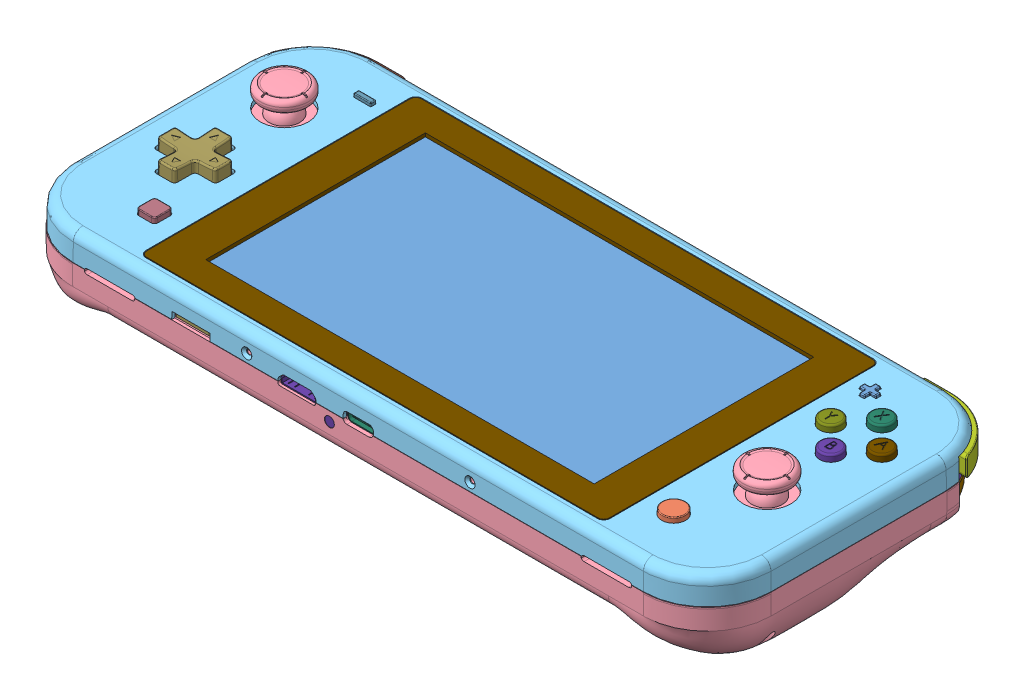
SolidWorks assembly Assembly Retro Lite CM5_1, configuration Default. Lengths in mm. (continued)
Components (placement in the parent): (continued)
- Assembly Center Components-1: Assembly Center Components [Default] at (0 9.4999 0) size (146.77 13.35 93.89) (continued)
  - Radxa CM3-1: Radxa CM3 [Default] at (-34.1679 -8.7691 -17.6603) x (0 0 -1) z (0 -1 0) size (40.05 55.02 3.7) (continued)
    - EMP_Models-1: EMP_Models [Default] at origin size (39.5 54.73 3.7) (continued)
      - C10-146: C10 [Default] at (-1.1975 3.8019 -1.2) x (-0.707107 -0.707107 0) z (0 0 -1) size (1.1 0.6 0.35)
      - C105-44: C105 [Default] at (-1.5975 -0.3481 -1.2) x (0.707107 0.707107 0) z (0 0 -1) size (2.5 1.3 0.6)
      - C10-147: C10 [Default] at (1.95 -3.55 -1.2) x (-0.707107 -0.707107 0) z (0 0 -1) size (1.1 0.6 0.35)
      - C10-148: C10 [Default] at (2.3 -3.9 -1.2) x (-0.707107 -0.707107 0) z (0 0 -1) size (1.1 0.6 0.35)
      - C10-149: C10 [Default] at (-1.7 4.85 -1.2) x (-0.707107 -0.707107 0) z (0 0 -1) size (1.1 0.6 0.35)
      - C10-150: C10 [Default] at (-0.45 4.65 -1.2) x (0.707107 -0.707107 0) z (0 0 -1) size (1.1 0.6 0.35)
      - C10-151: C10 [Default] at (-14.45 -16.6 -1.2) x (1 0 0) z (0 0 -1) size (1.1 0.6 0.35)
      - C10-152: C10 [Default] at (-5.6475 1.4519 -1.2) x (-0.707107 -0.707107 0) z (0 0 -1) size (1.1 0.6 0.35)
      - C10-153: C10 [Default] at (-9.5877 22.6017 0) x (0 1 0) z (0 0 1) size (1.1 0.6 0.35)
      - C10-154: C10 [Default] at (-4.9838 2.7384 -1.2) x (-0.707107 -0.707107 0) z (0 0 -1) size (1.1 0.6 0.35)
      - C10-155: C10 [Default] at (-3.4533 2.4614 -1.2) x (0.707107 0.707107 0) z (0 0 -1) size (1.1 0.6 0.35)
      - C10-156: C10 [Default] at (-4.2975 3.6019 -1.2) x (-0.707107 0.707107 0) z (0 0 -1) size (1.1 0.6 0.35)
      - C10-157: C10 [Default] at (1.6525 -1.6481 -1.2) x (-0.707107 -0.707107 0) z (0 0 -1) size (1.1 0.6 0.35)
      - C10-158: C10 [Default] at (0.25 10.55 -1.2) x (0 1 0) z (0 0 -1) size (1.1 0.6 0.35)
      - C10-159: C10 [Default] at (-5.2818 15.3952 0) size (1.1 0.6 0.35)
      - C10-160: C10 [Default] at (3.4025 -2.2481 -1.2) x (0.707107 0.707107 0) z (0 0 -1) size (1.1 0.6 0.35)
      - C10-161: C10 [Default] at (2.8025 -1.6481 -1.2) x (-0.707107 0.707107 0) z (0 0 -1) size (1.1 0.6 0.35)
      - C10-162: C10 [Default] at (-6.7675 7.1519 0) x (-0.707107 0.707107 0) z (0 0 1) size (1.1 0.6 0.35)
      - C10-163: C10 [Default] at (-6.3865 7.5329 0) x (-0.707107 0.707107 0) z (0 0 1) size (1.1 0.6 0.35)
      - C10-164: C10 [Default] at (8.6535 15.7139 -1.2) x (-1 0 0) z (0 0 -1) size (1.1 0.6 0.35)
      - C10-165: C10 [Default] at (-5.4975 8.5489 0) x (-0.707107 0.707107 0) z (0 0 1) size (1.1 0.6 0.35)
      - C10-166: C10 [Default] at (-5.9125 8.0719 0) x (-0.707107 0.707107 0) z (0 0 1) size (1.1 0.6 0.35)
      - C10-167: C10 [Default] at (-2.6475 4.9519 -1.2) x (0.707107 -0.707107 0) z (0 0 -1) size (1.1 0.6 0.35)
      - C1-22: C1 [Default] at (0.2025 -1.3981 -1.2) x (-0.707107 -0.707107 0) z (0 0 -1) size (1.7 0.9 0.5)
      - C10-168: C10 [Default] at (2.0525 -2.0981 -1.2) x (0.707107 0.707107 0) z (0 0 -1) size (1.1 0.6 0.35)
      - C1-23: C1 [Default] at (8.3303 14.9277 -1.2) x (-1 0 0) z (0 0 -1) size (1.7 0.9 0.5)
      - C1-24: C1 [Default] at (0.9 11.1 -1.2) x (0 1 0) z (0 0 -1) size (1.7 0.9 0.5)
      - C10-169: C10 [Default] at (-12.4547 0.1177 0) x (0.707107 -0.707107 0) z (0 0 1) size (1.1 0.6 0.35)
      - C10-170: C10 [Default] at (-12.9047 -0.3323 0) x (0.707107 -0.707107 0) z (0 0 1) size (1.1 0.6 0.35)
      - C10-171: C10 [Default] at (-6.4948 1.7665 -1.2) x (0.707107 -0.707107 0) z (0 0 -1) size (1.1 0.6 0.35)
      - C10-172: C10 [Default] at (-9.7716 0.8527 -1.2) x (-1 0 0) z (0 0 -1) size (1.1 0.6 0.35)
      - C10-173: C10 [Default] at (-7.95 1 -1.2) x (-0.707107 0.707107 0) z (0 0 -1) size (1.1 0.6 0.35)
      - C10-174: C10 [Default] at (-9.7407 -1.0384 -1.2) x (-1 0 0) z (0 0 -1) size (1.1 0.6 0.35)
      - C10-175: C10 [Default] at (-5.8561 -0.2604 -1.2) x (-0.707107 -0.707107 0) z (0 0 -1) size (1.1 0.6 0.35)
      - C1-25: C1 [Default] at (1.8025 -0.5481 -1.2) x (0.707107 0.707107 0) z (0 0 -1) size (1.7 0.9 0.5)
      - C10-176: C10 [Default] at (-5.0975 0.5019 -1.2) x (-0.707107 0.707107 0) z (0 0 -1) size (1.1 0.6 0.35)
      - C10-177: C10 [Default] at (2.5525 1.6519 -1.2) x (0.707107 0.707107 0) z (0 0 -1) size (1.1 0.6 0.35)
      - C10-178: C10 [Default] at (11.45 15.45 -1.2) x (0 1 0) z (0 0 -1) size (1.1 0.6 0.35)
      - C10-179: C10 [Default] at (2.7525 3.1519 -1.2) x (0.707107 0.707107 0) z (0 0 -1) size (1.1 0.6 0.35)
      - C10-180: C10 [Default] at (1.5525 2.5519 -1.2) x (0.707107 0.707107 0) z (0 0 -1) size (1.1 0.6 0.35)
      - C1-26: C1 [Default] at (13.7559 7.4017 0) size (1.7 0.9 0.5)
      - C10-181: C10 [Default] at (14.0564 10.6567 -1.2) x (0 1 0) z (0 0 -1) size (1.1 0.6 0.35)
      - C10-182: C10 [Default] at (14.055 9.1901 -1.2) x (0 -1 0) z (0 0 -1) size (1.1 0.6 0.35)
      - C10-183: C10 [Default] at (4.1525 -1.7481 -1.2) x (0.707107 -0.707107 0) z (0 0 -1) size (1.1 0.6 0.35)
      - C10-184: C10 [Default] at (2.0525 3.8519 -1.2) x (0.707107 0.707107 0) z (0 0 -1) size (1.1 0.6 0.35)
      - C1-27: C1 [Default] at (-0.4475 -0.7481 -1.2) x (-0.707107 -0.707107 0) z (0 0 -1) size (1.7 0.9 0.5)
      - C10-185: C10 [Default] at (-4.6 2.4 -1.2) x (-0.707107 -0.707107 0) z (0 0 -1) size (1.1 0.6 0.35)
      - C10-186: C10 [Default] at (2.4025 3.5019 -1.2) x (0.707107 0.707107 0) z (0 0 -1) size (1.1 0.6 0.35)
      - C10-187: C10 [Default] at (1.9025 2.2019 -1.2) x (0.707107 0.707107 0) z (0 0 -1) size (1.1 0.6 0.35)
      - C10-188: C10 [Default] at (1.1525 4.7519 -1.2) x (0.707107 0.707107 0) z (0 0 -1) size (1.1 0.6 0.35)
      - C10-189: C10 [Default] at (-10.8073 4.7134 0) x (-0.707107 0.707107 0) z (0 0 1) size (1.1 0.6 0.35)
      - C10-190: C10 [Default] at (-10.3573 5.1634 0) x (-0.707107 0.707107 0) z (0 0 1) size (1.1 0.6 0.35)
      - C10-191: C10 [Default] at (-9.9183 5.6024 0) x (-0.707107 0.707107 0) z (0 0 1) size (1.1 0.6 0.35)
      - C10-192: C10 [Default] at (-9.4886 6.0727 0) x (-0.707107 0.707107 0) z (0 0 1) size (1.1 0.6 0.35)
      - C10-193: C10 [Default] at (-8.5795 5.5319 0) x (-0.707107 0.707107 0) z (0 0 1) size (1.1 0.6 0.35)
      - C10-194: C10 [Default] at (-8.1985 5.9129 0) x (-0.707107 0.707107 0) z (0 0 1) size (1.1 0.6 0.35)
      - C105-45: C105 [Default] at (9.65 11.1 -1.2) x (-1 0 0) z (0 0 -1) size (2.5 1.3 0.6)
      - C10-195: C10 [Default] at (-7.2405 6.7439 0) x (-0.707107 0.707107 0) z (0 0 1) size (1.1 0.6 0.35)
      - C10-196: C10 [Default] at (-7.6905 6.2939 0) x (-0.707107 0.707107 0) z (0 0 1) size (1.1 0.6 0.35)
      - C10-197: C10 [Default] at (0.0606 6.505 -1.2) x (1 0 0) z (0 0 -1) size (1.1 0.6 0.35)
      - C10-198: C10 [Default] at (1.6025 4.3019 -1.2) x (0.707107 0.707107 0) z (0 0 -1) size (1.1 0.6 0.35)
      - C10-199: C10 [Default] at (0.45 4.15 -1.2) x (-0.707107 0.707107 0) z (0 0 -1) size (1.1 0.6 0.35)
      - C10-200: C10 [Default] at (4.3525 1.0519 -1.2) x (-0.707107 -0.707107 0) z (0 0 -1) size (1.1 0.6 0.35)
      - C10-201: C10 [Default] at (-0.25 3.6 -1.2) x (-0.707107 -0.707107 0) z (0 0 -1) size (1.1 0.6 0.35)
      - C10-202: C10 [Default] at (-4.7475 1.3019 -1.2) x (-0.707107 -0.707107 0) z (0 0 -1) size (1.1 0.6 0.35)
      - C10-203: C10 [Default] at (0.9 2.95 -1.2) x (0.707107 -0.707107 0) z (0 0 -1) size (1.1 0.6 0.35)
      - C10-204: C10 [Default] at (4.05 11.1 -1.2) x (0 -1 0) z (0 0 -1) size (1.1 0.6 0.35)
      - D1-1: D1 [Default] at (13.3703 9.2021 0) x (-1 0 0) z (0 0 1) size (3.3 1.4 0.8)
      - D1-2: D1 [Default] at (15.4253 4.4887 0) x (0 -1 0) z (0 0 1) size (3.3 1.4 0.8)
      - ED8144-1: ED8144 [Default] at (-15.7 3.95 0) x (0 1 0) z (0 0 1) size (1.77 0.93 0.8)
      - ED8144-2: ED8144 [Default] at (-14.65 -20.2 0) size (1.77 0.93 0.8)
      - ED8144-3: ED8144 [Default] at (-2.4887 24.0177 0) x (0 1 0) z (0 0 1) size (1.77 0.93 0.8)
      - ED8147-1: ED8147 [Default] at (18.2193 9.1971 0) size (2.41 1.24 0.8)
      - ED8144-4: ED8144 [Default] at (17.6586 1.0982 0) x (0 -1 0) z (0 0 1) size (1.77 0.93 0.8)
      - ED8144-5: ED8144 [Default] at (17.6586 2.8762 0) x (0 1 0) z (0 0 1) size (1.77 0.93 0.8)
      - FB1-1: FB1 [Default] at (1.65 9.65 -1.2) x (1 0 0) z (0 0 -1) size (1.7 0.8 0.5)
      - FB1-2: FB1 [Default] at (9.4715 23.3369 0) x (0 1 0) z (0 0 1) size (1.7 0.8 0.5)
      - FB1-3: FB1 [Default] at (10.7443 20.4739 -1.2) x (1 0 0) z (0 0 -1) size (1.7 0.8 0.5)
      - FB1-4: FB1 [Default] at (9.7417 13.5389 -1.2) x (1 0 0) z (0 0 -1) size (1.7 0.8 0.5)
      - FB1-5: FB1 [Default] at (12.05 13.95 -1.2) x (0 -1 0) z (0 0 -1) size (1.7 0.8 0.5)
      - FB1-6: FB1 [Default] at (3.5025 2.1519 -1.2) x (-0.707107 0.707107 0) z (0 0 -1) size (1.7 0.8 0.5)
      - FB5-1: FB5 [Default] at (17.7525 -10.7981 0) x (0 -1 0) z (0 0 1) size (2.08 1.34 0.7)
      - FB5-2: FB5 [Default] at (16.3025 -10.7981 0) x (0 -1 0) z (0 0 1) size (2.08 1.34 0.7)
      - FB5-3: FB5 [Default] at (14.8525 -10.7981 0) x (0 -1 0) z (0 0 1) size (2.08 1.34 0.7)
      - FB5-4: FB5 [Default] at (13.4025 -10.7981 0) x (0 -1 0) z (0 0 1) size (2.08 1.34 0.7)
      - FB9-1: FB9 [Default] at (11.1972 22.9552 0) size (2.8 1.3 0.6)
      - J1-1: J1 [Default] at (11.3212 22.5507 -1.2) x (0 1 0) z (0 0 -1) size (2.84 22.55 1)
      - J90033-1: J90033 [Default] at (-13.7 5.05 0) x (0 1 0) z (0 0 1) size (4.08 2.13 0.5)
      - J90033-2: J90033 [Default] at (-16.8 -18.5 0) x (-1 0 0) z (0 0 1) size (4.08 2.13 0.5)
      - L1-1: L1 [Default] at (9.3525 -25.5481 0) x (0 1 0) z (0 0 1) size (2.78 2.28 1)
      - L10-1: L10 [Default] at (5.8 11.7 0) x (0 1 0) z (0 0 1) size (2.78 2.28 1)
      - L10-2: L10 [Default] at (12.0115 18.7649 0) size (2.78 2.28 1)
      - L10-3: L10 [Default] at (-0.9 20.75 0) x (0 1 0) z (0 0 1) size (2.78 2.28 1)
      - L13-1: L13 [Default] at (-13.7665 -4.2312 0) x (-0.707107 -0.707107 0) z (0 0 1) size (2.83 2.1 1.2)
      - L2-1: L2 [Default] at (-11.1177 21.5067 0) x (-0.707107 -0.707107 0) z (0 0 1) size (1.1 0.6 0.35)
      - L2-2: L2 [Default] at (-11.7527 23.4117 0) x (-1 0 0) z (0 0 1) size (1.1 0.6 0.35)
      - L10-4: L10 [Default] at (-17.3475 4.7519 0) x (0 -1 0) z (0 0 1) size (2.78 2.28 1)
      - L10-5: L10 [Default] at (18.3025 -19.6481 0) x (-1 0 0) z (0 0 1) size (2.78 2.28 1)
      - L10-6: L10 [Default] at (9.2 12.15 0) x (-1 0 0) z (0 0 1) size (2.78 2.28 1)
      - L10-7: L10 [Default] at (-0.85 16.7 0) x (0 1 0) z (0 0 1) size (2.78 2.28 1)
      - LED1-1: LED1 [Default] at (-2.8224 26.4941 0) x (-1 0 0) z (0 0 1) size (2.95 1.43 0.6)
      - M1-1: M1 [Default] at (-12.0975 -25.5981 -1.2) x (-1 0 0) z (0 0 -1) size (3.45 3.45 0.1)
      - M1-2: M1 [Default] at (12.2025 25.6519 0) size (3.45 3.45 0.1)
      - M1-3: M1 [Default] at (-12.0975 -25.5981 0) size (3.45 3.45 0.1)
      - M1-4: M1 [Default] at (12.2025 25.6519 -1.2) x (-1 0 0) z (0 0 -1) size (3.45 3.45 0.1)
      - Q4-1: Q4 [Default] at (-8.45 5.5 -1.2) x (-1 0 0) z (0 0 -1) size (1.27 1.32 0.8)
      - Q5-1: Q5 [Default] at (-7.3 23.05 0) size (3.35 3.3 1)
      - Q5-2: Q5 [Default] at (17 -3.9 0) x (-1 0 0) z (0 0 1) size (3.35 3.3 1)
      - R1-1: R1 [Default] at (6.8025 -4.5481 -1.2) x (1 0 0) z (0 0 -1) size (1.7 0.9 0.5)
      - L2-3: L2 [Default] at (12.9303 4.6718 -1.2) x (0 -1 0) z (0 0 -1) size (1.1 0.6 0.35)
      - L2-4: L2 [Default] at (17.75 -11.3 -1.2) x (0 1 0) z (0 0 -1) size (1.1 0.6 0.35)
      - L2-5: L2 [Default] at (17.75 -12.45 -1.2) x (0 1 0) z (0 0 -1) size (1.1 0.6 0.35)
      - L2-6: L2 [Default] at (15.7025 -17.9981 -1.2) x (0 1 0) z (0 0 -1) size (1.1 0.6 0.35)
      - L2-7: L2 [Default] at (18.45 -11.3 -1.2) x (0 1 0) z (0 0 -1) size (1.1 0.6 0.35)
      - L2-8: L2 [Default] at (18.45 -12.45 -1.2) x (0 1 0) z (0 0 -1) size (1.1 0.6 0.35)
      - L2-9: L2 [Default] at (15.0525 -17.9981 -1.2) x (0 1 0) z (0 0 -1) size (1.1 0.6 0.35)
      - L2-10: L2 [Default] at (15.0525 -19.1481 -1.2) x (0 1 0) z (0 0 -1) size (1.1 0.6 0.35)
      - L2-11: L2 [Default] at (13.7525 -17.9981 -1.2) x (0 1 0) z (0 0 -1) size (1.1 0.6 0.35)
      - L2-12: L2 [Default] at (13.7525 -19.1481 -1.2) x (0 1 0) z (0 0 -1) size (1.1 0.6 0.35)
      - R1-2: R1 [Default] at (12.7025 -9.6481 0) size (1.7 0.9 0.5)
      - L2-13: L2 [Default] at (0.4486 12.9437 -1.2) x (0 1 0) z (0 0 -1) size (1.1 0.6 0.35)
      - R1-3: R1 [Default] at (13.1025 -8.2481 0) x (0 -1 0) z (0 0 1) size (1.7 0.9 0.5)
      - L2-14: L2 [Default] at (14.4025 -17.9981 -1.2) x (0 1 0) z (0 0 -1) size (1.1 0.6 0.35)
      - L2-15: L2 [Default] at (14.4025 -19.1481 -1.2) x (0 1 0) z (0 0 -1) size (1.1 0.6 0.35)
      - R1-4: R1 [Default] at (12.9525 -11.8481 -1.2) x (-1 0 0) z (0 0 -1) size (1.7 0.9 0.5)
      - R1-5: R1 [Default] at (18.8525 -19.1481 -1.2) x (-1 0 0) z (0 0 -1) size (1.7 0.9 0.5)
      - L2-16: L2 [Default] at (11.8525 -13.8481 -1.2) x (0 -1 0) z (0 0 -1) size (1.1 0.6 0.35)
      - L2-17: L2 [Default] at (11.6025 -15.0981 -1.2) x (1 0 0) z (0 0 -1) size (1.1 0.6 0.35)
      - L2-18: L2 [Default] at (11.2025 -13.8481 -1.2) x (0 -1 0) z (0 0 -1) size (1.1 0.6 0.35)
      - L2-19: L2 [Default] at (11.7525 -16.2481 -1.2) x (-1 0 0) z (0 0 -1) size (1.1 0.6 0.35)
      - L2-20: L2 [Default] at (13.9025 -20.1981 0) x (0 -1 0) z (0 0 1) size (1.1 0.6 0.35)
      - R1-6: R1 [Default] at (11.8808 6.1274 0) size (1.7 0.9 0.5)
      - R1-7: R1 [Default] at (10.5014 7.0239 0) x (0 1 0) z (0 0 1) size (1.7 0.9 0.5)
      - L2-21: L2 [Default] at (-10.0048 -2.9217 0) x (-1 0 0) z (0 0 1) size (1.1 0.6 0.35)
      - L2-22: L2 [Default] at (-11.25 4.25 0) x (-0.707107 0.707107 0) z (0 0 1) size (1.1 0.6 0.35)
      - L2-23: L2 [Default] at (-7.55 2.1989 -1.2) x (1 0 0) z (0 0 -1) size (1.1 0.6 0.35)
      - L2-24: L2 [Default] at (18.2 -17.4 -1.2) x (-1 0 0) z (0 0 -1) size (1.1 0.6 0.35)
      - L2-25: L2 [Default] at (18.2 -16.75 -1.2) x (-1 0 0) z (0 0 -1) size (1.1 0.6 0.35)
      - L2-26: L2 [Default] at (19.25 -17.15 -1.2) x (0 -1 0) z (0 0 -1) size (1.1 0.6 0.35)
      - L2-27: L2 [Default] at (-13.3547 0.5177 0) x (-0.707107 -0.707107 0) z (0 0 1) size (1.1 0.6 0.35)
      - L2-28: L2 [Default] at (-3.95 9.75 0) x (0.707107 0.707107 0) z (0 0 1) size (1.1 0.6 0.35)
      - L2-29: L2 [Default] at (-7.45 4.9 -1.2) x (0 1 0) z (0 0 -1) size (1.1 0.6 0.35)
      - L2-30: L2 [Default] at (-3.35 10.8 0) x (0 1 0) z (0 0 1) size (1.1 0.6 0.35)
      - L2-31: L2 [Default] at (-8.9 -1.05 -1.2) x (0 1 0) z (0 0 -1) size (1.1 0.6 0.35)
      - L2-32: L2 [Default] at (-9.7407 -0.3884 -1.2) x (-1 0 0) z (0 0 -1) size (1.1 0.6 0.35)
      - L2-33: L2 [Default] at (1.5025 -5.4481 -1.2) x (-0.707107 -0.707107 0) z (0 0 -1) size (1.1 0.6 0.35)
      - L2-34: L2 [Default] at (-9.7625 1.3757 -1.2) x (1 0 0) z (0 0 -1) size (1.1 0.6 0.35)
      - L2-35: L2 [Default] at (-9.7722 0.251 -1.2) x (1 0 0) z (0 0 -1) size (1.1 0.6 0.35)
      - L2-36: L2 [Default] at (8.8525 -3.8481 -1.2) x (1 0 0) z (0 0 -1) size (1.1 0.6 0.35)
      - L2-37: L2 [Default] at (8.8525 -4.4981 -1.2) x (1 0 0) z (0 0 -1) size (1.1 0.6 0.35)
      - R24-1: R24 [Default] at (13.5019 5.7507 0) x (0 -1 0) z (0 0 1) size (2.5 1.3 0.6)
      - L2-38: L2 [Default] at (8.8525 -5.1481 -1.2) x (1 0 0) z (0 0 -1) size (1.1 0.6 0.35)
      - R1-8: R1 [Default] at (11.8808 7.9054 0) x (-1 0 0) z (0 0 1) size (1.7 0.9 0.5)
      - L2-39: L2 [Default] at (8.839 -5.6572 -1.2) x (-1 0 0) z (0 0 -1) size (1.1 0.6 0.35)
      - L2-40: L2 [Default] at (13.5019 8.1637 0) size (1.1 0.6 0.35)
      - R1-9: R1 [Default] at (11.8808 7.0164 0) x (-1 0 0) z (0 0 1) size (1.7 0.9 0.5)
      - L2-41: L2 [Default] at (1.9025 -4.5981 -1.2) x (-0.707107 0.707107 0) z (0 0 -1) size (1.1 0.6 0.35)
      - R1-10: R1 [Default] at (12.4 10.2 -1.2) x (-1 0 0) z (0 0 -1) size (1.7 0.9 0.5)
      - R1-11: R1 [Default] at (12.4278 9.235 -1.2) x (-1 0 0) z (0 0 -1) size (1.7 0.9 0.5)
      - L2-42: L2 [Default] at (0.0025 12.7519 0) x (0.707107 0.707107 0) z (0 0 1) size (1.1 0.6 0.35)
      - L2-43: L2 [Default] at (0.4393 12.3013 0) x (0.707107 0.707107 0) z (0 0 1) size (1.1 0.6 0.35)
      - L2-44: L2 [Default] at (0.9525 11.8019 0) x (0.707107 0.707107 0) z (0 0 1) size (1.1 0.6 0.35)
      - L2-45: L2 [Default] at (1.3881 11.3747 0) x (0.707107 0.707107 0) z (0 0 1) size (1.1 0.6 0.35)
      - L2-46: L2 [Default] at (1.9025 10.8519 0) x (0.707107 0.707107 0) z (0 0 1) size (1.1 0.6 0.35)
      - L2-47: L2 [Default] at (2.3296 10.4351 0) x (0.707107 0.707107 0) z (0 0 1) size (1.1 0.6 0.35)
      - L2-48: L2 [Default] at (2.8525 9.9019 0) x (0.707107 0.707107 0) z (0 0 1) size (1.1 0.6 0.35)
      - L2-49: L2 [Default] at (3.2748 9.4731 0) x (0.707107 0.707107 0) z (0 0 1) size (1.1 0.6 0.35)
      - L2-50: L2 [Default] at (-4.75 10.35 0) x (-1 0 0) z (0 0 1) size (1.1 0.6 0.35)
      - L2-51: L2 [Default] at (1.1909 6.5961 -1.2) x (0 -1 0) z (0 0 -1) size (1.1 0.6 0.35)
      - L2-52: L2 [Default] at (10.3525 2.1019 0) x (-0.707107 0.707107 0) z (0 0 1) size (1.1 0.6 0.35)
      - R1-12: R1 [Default] at (9.9432 9.4653 0) size (1.7 0.9 0.5)
      - R1-13: R1 [Default] at (9.5622 8.0683 0) x (0 -1 0) z (0 0 1) size (1.7 0.9 0.5)
      - L2-53: L2 [Default] at (-8.7065 -3.7391 0) size (1.1 0.6 0.35)
      - L2-54: L2 [Default] at (-8.7065 -4.3741 0) size (1.1 0.6 0.35)
      - L2-55: L2 [Default] at (-6.5975 -2.9981 -1.2) x (-0.707107 -0.707107 0) z (0 0 -1) size (1.1 0.6 0.35)
      - R1-14: R1 [Default] at (-15.4372 0.8153 0) x (-1 0 0) z (0 0 1) size (1.7 0.9 0.5)
      - L2-56: L2 [Default] at (-18.76 -2.973 0) x (-0.707107 0.707107 0) z (0 0 1) size (1.1 0.6 0.35)
      - R1-15: R1 [Default] at (-15.0359 2.0509 0) x (0 1 0) z (0 0 1) size (1.7 0.9 0.5)
      - L2-57: L2 [Default] at (-5.15 9.75 0) x (-1 0 0) z (0 0 1) size (1.1 0.6 0.35)
      - L2-58: L2 [Default] at (-18.3381 -2.5736 0) x (0.707107 -0.707107 0) z (0 0 1) size (1.1 0.6 0.35)
      - L2-59: L2 [Default] at (5.8025 -20.8481 -1.2) x (1 0 0) z (0 0 -1) size (1.1 0.6 0.35)
      - L2-60: L2 [Default] at (5.8025 -20.1981 -1.2) x (1 0 0) z (0 0 -1) size (1.1 0.6 0.35)
      - R24-2: R24 [Default] at (11.9025 -23.7981 -1.2) x (-1 0 0) z (0 0 -1) size (2.5 1.3 0.6)
      - R1-16: R1 [Default] at (-13.55 -21.25 -1.2) x (1 0 0) z (0 0 -1) size (1.7 0.9 0.5)
      - R24-3: R24 [Default] at (7.0025 -26.5481 -1.2) x (-1 0 0) z (0 0 -1) size (2.5 1.3 0.6)
      - R1-17: R1 [Default] at (-13.55 -20.3 -1.2) x (1 0 0) z (0 0 -1) size (1.7 0.9 0.5)
      - L2-61: L2 [Default] at (11.5525 -21.7481 0) size (1.1 0.6 0.35)
      - L2-62: L2 [Default] at (12.7525 -26.2481 -1.2) x (1 0 0) z (0 0 -1) size (1.1 0.6 0.35)
      - L2-63: L2 [Default] at (-18.4 -16.6 -1.2) x (1 0 0) z (0 0 -1) size (1.1 0.6 0.35)
      - L2-64: L2 [Default] at (-1.6 13.75 0) x (0 1 0) z (0 0 1) size (1.1 0.6 0.35)
      - L2-65: L2 [Default] at (13.9525 -26.8981 0) size (1.1 0.6 0.35)
      - L2-66: L2 [Default] at (-12.014 6.1193 -1.2) x (0 1 0) z (0 0 -1) size (1.1 0.6 0.35)
      - L2-67: L2 [Default] at (-10.4 5.9 -1.2) x (0 1 0) z (0 0 -1) size (1.1 0.6 0.35)
      - L2-68: L2 [Default] at (-12.6417 6.1168 -1.2) x (0 1 0) z (0 0 -1) size (1.1 0.6 0.35)
      - L2-69: L2 [Default] at (-11.4087 6.1174 -1.2) x (0 1 0) z (0 0 -1) size (1.1 0.6 0.35)
      - L2-70: L2 [Default] at (-12.6469 -1.643 -1.2) x (1 0 0) z (0 0 -1) size (1.1 0.6 0.35)
      - L2-71: L2 [Default] at (13.1198 7.7736 -1.2) x (1 0 0) z (0 0 -1) size (1.1 0.6 0.35)
      - L2-72: L2 [Default] at (-16.9 -11.65 -1.2) x (-1 0 0) z (0 0 -1) size (1.1 0.6 0.35)
      - L2-73: L2 [Default] at (-18.1 -11.65 -1.2) x (1 0 0) z (0 0 -1) size (1.1 0.6 0.35)
      - L2-74: L2 [Default] at (-15.6 -15.95 -1.2) x (-1 0 0) z (0 0 -1) size (1.1 0.6 0.35)
      - L2-75: L2 [Default] at (-12.55 0.45 -1.2) x (-1 0 0) z (0 0 -1) size (1.1 0.6 0.35)
      - L2-76: L2 [Default] at (-13.55 0.45 -1.2) x (-1 0 0) z (0 0 -1) size (1.1 0.6 0.35)
      - R24-4: R24 [Default] at (-14.4732 17.1388 -1.2) x (0 1 0) z (0 0 -1) size (2.5 1.3 0.6)
      - L2-77: L2 [Default] at (-17.707 19.6733 -1.2) x (1 0 0) z (0 0 -1) size (1.1 0.6 0.35)
      - L2-78: L2 [Default] at (13.1107 8.3605 -1.2) x (1 0 0) z (0 0 -1) size (1.1 0.6 0.35)
      - L2-79: L2 [Default] at (-17.7116 19.1714 -1.2) x (-1 0 0) z (0 0 -1) size (1.1 0.6 0.35)
      - L2-80: L2 [Default] at (-12.999 2.1325 0) x (-1 0 0) z (0 0 1) size (1.1 0.6 0.35)
      - L2-81: L2 [Default] at (-5.9125 16.7079 0) x (0 1 0) z (0 0 1) size (1.1 0.6 0.35)
      - L2-82: L2 [Default] at (-18.8975 5.2019 0) x (0 -1 0) z (0 0 1) size (1.1 0.6 0.35)
      - R1-18: R1 [Default] at (-17.0263 0.7967 0) size (1.7 0.9 0.5)
      - R1-19: R1 [Default] at (-16.2916 2.0337 0) x (0 1 0) z (0 0 1) size (1.7 0.9 0.5)
      - L2-83: L2 [Default] at (-11.7975 6.8019 0) size (1.1 0.6 0.35)
      - L2-84: L2 [Default] at (18.85 -12.45 0) size (1.1 0.6 0.35)
      - L2-85: L2 [Default] at (18.85 -11.8 0) size (1.1 0.6 0.35)
      - L2-86: L2 [Default] at (12.2953 4.6718 -1.2) x (0 -1 0) z (0 0 -1) size (1.1 0.6 0.35)
      - L2-87: L2 [Default] at (18.85 -13.1 0) size (1.1 0.6 0.35)
      - L2-88: L2 [Default] at (18.1 -0.6 0) x (0 1 0) z (0 0 1) size (1.1 0.6 0.35)
      - L2-89: L2 [Default] at (17.45 -0.6 0) x (0 1 0) z (0 0 1) size (1.1 0.6 0.35)
      - L2-90: L2 [Default] at (18.2 -15.45 -1.2) x (1 0 0) z (0 0 -1) size (1.1 0.6 0.35)
      - L2-91: L2 [Default] at (9.0525 1.2019 -1.2) x (-1 0 0) z (0 0 -1) size (1.1 0.6 0.35)
      - L2-92: L2 [Default] at (-10.2001 3.3697 -1.2) x (0 1 0) z (0 0 -1) size (1.1 0.6 0.35)
      - L2-93: L2 [Default] at (-16.15 -20.2 0) size (1.1 0.6 0.35)
      - R24-5: R24 [Default] at (-8.1 25.45 0) x (-1 0 0) z (0 0 1) size (2.5 1.3 0.6)
      - L2-94: L2 [Default] at (11.7 13.4 0) x (0 1 0) z (0 0 1) size (1.1 0.6 0.35)
      - L2-95: L2 [Default] at (3.95 11.85 0) x (-1 0 0) z (0 0 1) size (1.1 0.6 0.35)
      - L2-96: L2 [Default] at (10.8685 18.0306 -1.2) x (-1 0 0) z (0 0 -1) size (1.1 0.6 0.35)
      - L2-97: L2 [Default] at (8.5825 18.5109 -1.2) x (-1 0 0) z (0 0 -1) size (1.1 0.6 0.35)
      - L2-98: L2 [Default] at (5.9323 23.8177 0) x (0 -1 0) z (0 0 1) size (1.1 0.6 0.35)
      - L2-99: L2 [Default] at (5.2823 23.8177 0) x (0 -1 0) z (0 0 1) size (1.1 0.6 0.35)
      - L2-100: L2 [Default] at (-8.8 24.55 0) x (-1 0 0) z (0 0 1) size (1.1 0.6 0.35)
      - R9216-1: R9216 [Default] at (3.3 18.2 -1.2) x (1 0 0) z (0 0 -1) size (3.6 2.1 0.8)
      - L2-101: L2 [Default] at (-0.3818 13.9135 -1.2) x (0 1 0) z (0 0 -1) size (1.1 0.6 0.35)
      - L2-102: L2 [Default] at (0.45 16.7 -1.2) x (-1 0 0) z (0 0 -1) size (1.1 0.6 0.35)
      - L2-103: L2 [Default] at (-0.3818 14.9291 -1.2) x (0 1 0) z (0 0 -1) size (1.1 0.6 0.35)
      - L2-104: L2 [Default] at (0.55 14.45 -1.2) x (-1 0 0) z (0 0 -1) size (1.1 0.6 0.35)
      - L2-105: L2 [Default] at (-1.1 14.15 0) x (0 -1 0) z (0 0 1) size (1.1 0.6 0.35)
      - L2-106: L2 [Default] at (0.75 14.6 0) x (0 1 0) z (0 0 1) size (1.1 0.6 0.35)
      - L2-107: L2 [Default] at (-3.9887 23.8177 0) x (0 1 0) z (0 0 1) size (1.1 0.6 0.35)
      - R9216-2: R9216 [Default] at (16.5683 7.4937 0) x (-1 0 0) z (0 0 1) size (3.6 2.1 0.8)
      - L2-108: L2 [Default] at (-18.0618 -3.6891 0) x (0.707107 -0.707107 0) z (0 0 1) size (1.1 0.6 0.35)
      - L2-109: L2 [Default] at (-16.8694 -1.2155 0) x (-0.707107 -0.707107 0) z (0 0 1) size (1.1 0.6 0.35)
      - L2-110: L2 [Default] at (-18.4855 -4.1201 0) x (0.707107 -0.707107 0) z (0 0 1) size (1.1 0.6 0.35)
      - R1-20: R1 [Default] at (4.2 12.6 -1.2) x (0 1 0) z (0 0 -1) size (1.7 0.9 0.5)
      - R1-21: R1 [Default] at (2.6 12.6 -1.2) x (0 1 0) z (0 0 -1) size (1.7 0.9 0.5)
      - R1-22: R1 [Default] at (5 12.6 -1.2) x (0 1 0) z (0 0 -1) size (1.7 0.9 0.5)
      - R1-23: R1 [Default] at (9.8 14.3 -1.2) x (-1 0 0) z (0 0 -1) size (1.7 0.9 0.5)
      - R1-24: R1 [Default] at (-18.35 1.2 0) x (0 1 0) z (0 0 1) size (1.7 0.9 0.5)
      - R1-25: R1 [Default] at (3.4 12.6 -1.2) x (0 1 0) z (0 0 -1) size (1.7 0.9 0.5)
      - L2-111: L2 [Default] at (-3.1812 25.4157 0) size (1.1 0.6 0.35)
      - L2-112: L2 [Default] at (15.7205 1.3062 0) size (1.1 0.6 0.35)
      - L2-113: L2 [Default] at (15.7205 1.9412 0) size (1.1 0.6 0.35)
      - L2-114: L2 [Default] at (14.7219 1.3075 0) x (-1 0 0) z (0 0 1) size (1.1 0.6 0.35)
      - L2-115: L2 [Default] at (14.9 -3.05 0) x (0 -1 0) z (0 0 1) size (1.1 0.6 0.35)
      - L2-116: L2 [Default] at (17.7 -1.55 0) size (1.1 0.6 0.35)
      - L2-117: L2 [Default] at (-7.95 26.5 0) x (-1 0 0) z (0 0 1) size (1.1 0.6 0.35)
      - L2-118: L2 [Default] at (-9 1.15 -1.2) x (0 1 0) z (0 0 -1) size (1.1 0.6 0.35)
      - L2-119: L2 [Default] at (17.5 -14.2 -1.2) x (-1 0 0) z (0 0 -1) size (1.1 0.6 0.35)
      - L2-120: L2 [Default] at (13.1025 -19.1481 -1.2) x (0 1 0) z (0 0 -1) size (1.1 0.6 0.35)
      - L2-121: L2 [Default] at (19.15 -11.3 -1.2) x (0 1 0) z (0 0 -1) size (1.1 0.6 0.35)
      - L2-122: L2 [Default] at (19.15 -12.45 -1.2) x (0 1 0) z (0 0 -1) size (1.1 0.6 0.35)
      - L2-123: L2 [Default] at (18.7525 -17.9981 0) size (1.1 0.6 0.35)
      - L2-124: L2 [Default] at (15.2025 -20.1981 0) x (0 -1 0) z (0 0 1) size (1.1 0.6 0.35)
      - L2-125: L2 [Default] at (14.0025 -20.0481 -1.2) x (1 0 0) z (0 0 -1) size (1.1 0.6 0.35)
      - TP1-1: TP1 [Default] at (-12.0342 7.0446 -1.2) x (-1 0 0) z (0 0 -1) size (1 1 0.1)
      - TP1-2: TP1 [Default] at (18.7 0.35 0) size (1 1 0.1)
      - TP1-3: TP1 [Default] at (-7 3 -1.2) x (-0.707107 0.707107 0) z (0 0 -1) size (1 1 0.1)
      - TP1-4: TP1 [Default] at (18.75 13.45 -1.2) x (-1 0 0) z (0 0 -1) size (1 1 0.1)
      - TP1-5: TP1 [Default] at (19.4 9.05 -1.2) x (-1 0 0) z (0 0 -1) size (1 1 0.1)
      - TP1-6: TP1 [Default] at (19.4 10.6 -1.2) x (-1 0 0) z (0 0 -1) size (1 1 0.1)
      - TP1-7: TP1 [Default] at (-18.6 -15.75 -1.2) x (-1 0 0) z (0 0 -1) size (1 1 0.1)
      - TP1-8: TP1 [Default] at (-17.5 -15.75 -1.2) x (-1 0 0) z (0 0 -1) size (1 1 0.1)
      - TP1-9: TP1 [Default] at (14.35 -10.85 -1.2) x (-1 0 0) z (0 0 -1) size (1 1 0.1)
      - TP1-10: TP1 [Default] at (-8.8451 3.2927 -1.2) x (-1 0 0) z (0 0 -1) size (1 1 0.1)
      - TP1-11: TP1 [Default] at (4.5413 20.3907 -1.2) x (-1 0 0) z (0 0 -1) size (1 1 0.1)
      - TP1-12: TP1 [Default] at (18.6825 1.3989 0) size (1 1 0.1)
      - TP1-13: TP1 [Default] at (18.6825 2.4489 0) size (1 1 0.1)
      - U1-1: U1 [Default] at (-0.1975 0.4519 0) x (-0.707107 0.707107 0) z (0 0 1) size (18.71 17.21 1.1)
      - U2-1: U2 [Default] at (-1.0248 -19.8218 0) x (0 -1 0) z (0 0 1) size (13.49 18.53 1)
      - U3-1: U3 [Default] at (12.9025 -23.7481 0) x (0 -1 0) z (0 0 1) size (4.03 3.13 1)
      - U3-2: U3 [Default] at (-18.15 -19.4 -1.2) x (1 0 0) z (0 0 -1) size (4.03 3.13 1)
      - U4300-1: U4300 [Default] at (-16.9 -13.45 0) x (-1 0 0) z (0 0 1) size (5.99 7 1.2)
      - U4301-1: U4301 [Default] at (5.2805 18.1299 0) x (0 1 0) z (0 0 1) size (8.35 8.35 0.8)
      - U4302-1: U4302 [Default] at (-16.4535 -5.0091 0) x (0.707107 0.707107 0) z (0 0 1) size (1.93 2.38 0.8)
      - U5-1: U5 [Default] at (-7.6975 14.2519 -1.2) x (1 0 0) z (0 0 -1) size (11.63 13.5 1.2)
      - U7-1: U7 [Default] at (14.2608 3.741 0) x (0 -1 0) z (0 0 1) size (2.08 2.45 0.7)
      - U8-1: U8 [Default] at (-12.9975 13.9519 0) x (0 -1 0) z (0 0 1) size (13.66 12.7 1.3)
      - U9-1: U9 [Default] at (15.3025 -15.6981 0) x (0 -1 0) z (0 0 1) size (5.84 5.5 1)
      - U3-3: U3 [Default] at (13.5 0.3 0) size (4.03 3.13 1)
      - Y1-1: Y1 [Default] at (-4.2838 13.1005 0) x (-1 0 0) z (0 0 1) size (3.6 3.57 1.2)
      - Y1-2: Y1 [Default] at (-17.6116 16.6641 -1.2) x (-1 0 0) z (0 0 -1) size (3.6 3.57 1.2)
      - Y1-3: Y1 [Default] at (17.8 -7.6 0) x (0 -1 0) z (0 0 1) size (3.6 3.57 1.2)
      - Y4-1: Y4 [Default] at (-0.81 24.6548 0) size (3.6 1.7 1.2)
    - Board_outline(1)-1: Board_outline(1) [Default] at origin size (40.05 55.02 1.2)
  - User Library-CR1225 v1-1: User Library-CR1225 v1 [Default] at (-65.8849 -7.0512 19.9145) x (0 0 -1) z (0 -1 0) size (12.4 12.4 2.5)
    - refine_Revolution001-1: refine_Revolution001 [Default] at (0 0 2.5) x (1 0 0) z (0 1 0) size (10.2 0.85 10.2)
    - refine_Cut001-1: refine_Cut001 [Default] at (0 1 2.5) x (1 0 0) z (0 1 0) size (12.4 2.5 12.4)
  - 5040500491 v1-1: 5040500491 v1 [Default] at (-31.1609 -7.15 36.6709) x (-1 0 0) z (0 -1 0) size (10.55 6.44 2)
    - 5040500491-1: 5040500491 [Default] at origin size (10.55 6.44 2)
  - DF40C-100DS-1: DF40C-100DS [Default] at (-37.655 -6.2 -0.495) x (0 0 -1) z (-1 0 0) size (3.49 2 22.61)
  - DF40C-100DS-2: DF40C-100DS [Default] at (-37.655 -6.2 -34.495) x (0 0 -1) z (-1 0 0) size (3.49 2 22.61)
  - Micro SD-Card-1: Micro SD-Card [Default] at (-52.45 -7.1 39.52) x (0 0 -1) z (-1 0 0) size (15 1.01 11)
  - CUI_DEVICES_SJ-43516-SMT-TR-1: CUI_DEVICES_SJ-43516-SMT-TR [Default] at (-2.55 -8.65 -45.17) x (0 0 -1) z (-1 0 0) size (19.2 5.8 9)
  - PCIe Slot  v1-1: PCIe Slot  v1 [Default] at (-9.09 -6.1502 6.7) x (-1 0 0) z (0 0 1) size (22 4.8 8.55)
  - 1054500101 v1-1: 1054500101 v1 [Default] at (0 -7.7798 41.669) x (1 0 0) z (0 -1 0) size (8.94 7.9 3.96)
  - 502570-0893 v1-1: 502570-0893 v1 [Default] at (-97.1844 -7.0502 -24.8743) x (1 0 0) z (0 -1 0) size (13.8 15.5 1.8)
  - 9774025243R (rev1) v1-1: 9774025243R (rev1) v1 [Default] at (0 -52.8238 2.1762) x (1 0 0) z (0 -1 0) size (4.35 4.35 3.9)
  - DF40C-100DS-3: DF40C-100DS [Default] at (-9.8603 -6.2 -23.511) x (1 0 0) z (0 0 -1) size (3.49 2 22.61)
  - 5051100892 v1-1: 5051100892 v1 [Default] at (-65.4404 -6.1942 -19.6945) x (0 0 1) z (1 0 0) size (9.5 1.9 5.3)
  - keystone-PN1072TR v1-1: keystone-PN1072TR v1 [Default] at (-72.6801 -0.2846 31.6836) x (1 0 0) z (0 0 -1) size (10.39 4.4 15.9)
  - TPS65987DDHRSHR--3DModel-STEP-56544 v1-1: TPS65987DDHRSHR--3DModel-STEP-56544 v1 [Default] at (-12.5607 -6.1 22.9561) x (-1 0 0) z (0 0 1) size (7 1 7)
  - TPD4E05U06DQAR--3DModel-STEP-56544 v1-1: TPD4E05U06DQAR--3DModel-STEP-56544 v1 [Default] at (4.7671 -6.1 32.9073) x (0 0 1) z (1 0 0) size (1 0.55 2.5)
  - TPD4E05U06DQAR--3DModel-STEP-56544 v1-2: TPD4E05U06DQAR--3DModel-STEP-56544 v1 [Default] at (-3.01 -6.1 32.9073) x (0 0 1) z (1 0 0) size (1 0.55 2.5)
  - TSIC 306 SOP-8--3DModel-STEP-510211 v1-1: TSIC 306 SOP-8--3DModel-STEP-510211 v1 [Default] at (-60.1923 -6.1499 6.8931) x (-1 0 0) z (0 0 1) size (5.99 1.73 4.93)
  - 5034801700 v1-1: 5034801700 v1 [Default] at (6.9127 -6.1711 10.2732) x (0 0 1) z (1 0 0) size (10.2 1.87 3.6)
  - 5034801700 v1-2: 5034801700 v1 [Default] at (-25.1264 -6.1711 10.2943) x (0 0 -1) z (-1 0 0) size (10.2 1.87 3.6)
  - VLCF4020T-220MR56--3DModel-STEP-56544 v1-1: VLCF4020T-220MR56--3DModel-STEP-56544 v1 [Default] at (-60.5998 -6.1052 -39.9462) x (0 0 -1) z (-1 0 0) size (4 2.02 4.05)
  - Heatsink-V2 v1-1: Heatsink-V2 v1 [Default] at (-21.2372 -13.3527 3.8484) x (0 0 -1) z (1 0 0) size (46.85 6 53)
  - QFN_GEFLRV_CIR v1-1: QFN_GEFLRV_CIR v1 [Default] at (0.5729 -5.758 -18.9632) x (1 0 0) z (0 -1 0) size (5 5 0.99)
  - 505110-3091 v1-1: 505110-3091 v1 [Default] at (-70.5178 -6.0871 -0.2937) x (0 0 1) z (1 0 0) size (20.5 1.9 5.3)
  - ASPI-0630HI v1-1: ASPI-0630HI v1 [Default] at (-31.1721 -7.6525 20.8058) x (-1 0 0) z (0 0 1) size (7.2 3 6.65)
  - Retro Lite CM5 (Latest)-18-1: Retro Lite CM5 (Latest)-18 [Default] at origin size (60.98 9.58 0.4)
  - Retro Lite CM5 Carrier Board_CM5IO_Mapping_X2.0 v3-1: Retro Lite CM5 Carrier Board_CM5IO_Mapping_X2.0 v3 [Default] at (-1.05 -5.1782 42.5) x (-1 0 0) z (0 -1 0) size (82.67 91.25 0.97)
    - Retro Lite CM5 Carrier Board_CM5IO_Mapping_X2.0 v3(2)^Retro Lite CM5 Carrier Board_CM5IO_Mapping_X2.0 v3-1: Retro Lite CM5 Carrier Board_CM5IO_Mapping_X2.0 v3(2)^Retro Lite CM5 Carrier Board_CM5IO_Mapping_X2.0 v3 [Default] at origin size (82.67 91.25 0.97) (virtual)
      - Board^Retro Lite CM5 Carrier Board_CM5IO_Mapping_X2.0 v3(2)_Retro Lite CM5 Carrier Board_CM5IO_Mapping_X2.0 v3-1: Board^Retro Lite CM5 Carrier Board_CM5IO_Mapping_X2.0 v3(2)_Retro Lite CM5 Carrier Board_CM5IO_Mapping_X2.0 v3 [Default] at origin size (82.67 91.25 0.97) (virtual)
